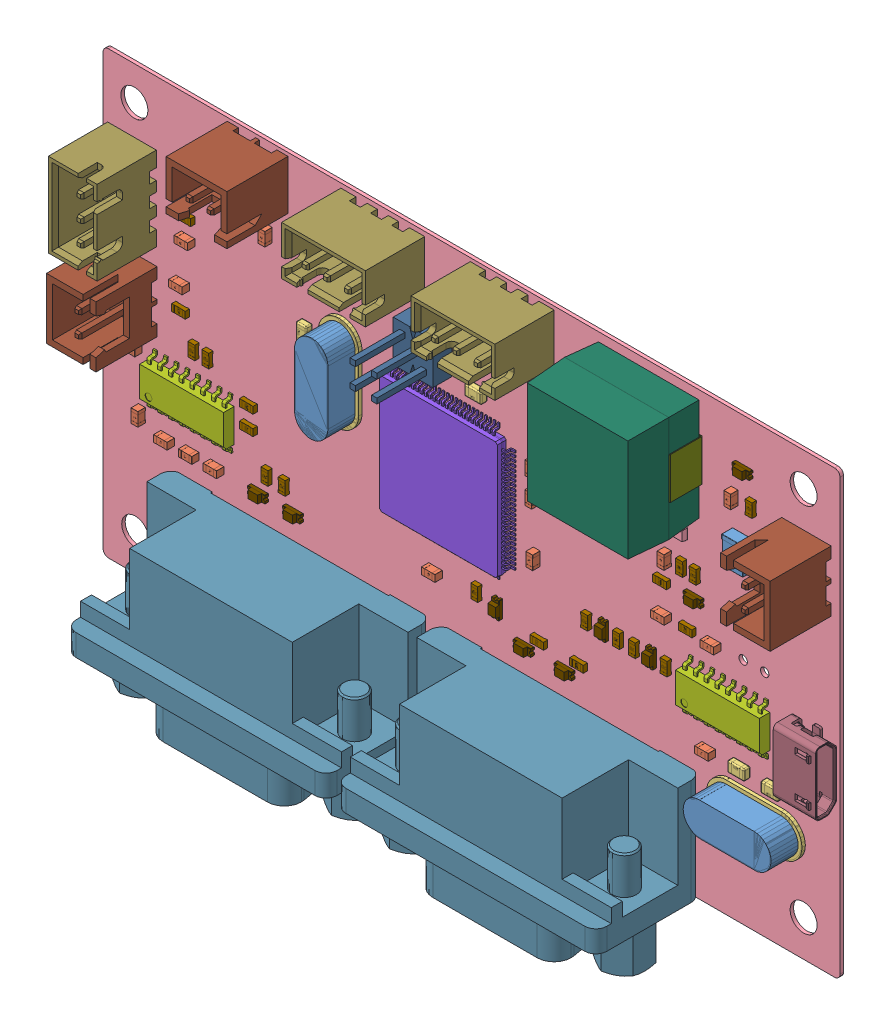
SolidWorks assembly Motor_Driver_Module, configuration Default. Lengths in mm.
Overall size (87 57.49 16.88).
208 component instances, 22 part files, 0 mates.
Components (placement in the parent):
- Motor_Driver_Module.step-1: Motor_Driver_Module.step [Default] at origin size (87 57.49 16.88)
  - X2.step-1: X2.step [Default] at origin size (11.27 4.77 5.6)
    - Xtal2.step-1: Xtal2.step [Default] at (353.2221 89.0021 0) x (-1 0 0) z (0 0 1) size (11.17 4.67 5.6)
      - User_Library-HC49S_Open_CASCADE_STEP_translator_6.2_316.2.step-1: User_Library-HC49S_Open_CASCADE_STEP_translator_6.2_316.2.step [Default] at origin size (11.17 4.67 5.6)
        - User_Library-HC49S_HC49S1.step-1: User_Library-HC49S_HC49S1.step [Default] at (0 0.0112 0.0127) size (11.17 4.67 5.6)
          - User_Library-HC49S_Open_CASCADE_STEP_translator_6.2_282.2.step-1: User_Library-HC49S_Open_CASCADE_STEP_translator_6.2_282.2.step [Default] at origin size (11.17 4.67 5.6)
            - User_Library-HC49S_340979409.step-1: User_Library-HC49S_340979409.step [Default] at (2.575 0.0126 0.0127) size (10.27 3.84 3.6)
              - User_Library-HC49S_Extruded3.step-1: User_Library-HC49S_Extruded3.step [Default] at origin size (10.27 3.84 3.6)
            - User_Library-HC49S_340739185.step-1: User_Library-HC49S_340739185.step [Default] at (-0.0117 -0.0104 -1.9873) size (0.43 0.43 2.1)
              - User_Library-HC49S_Cylinder1.step-1: User_Library-HC49S_Cylinder1.step [Default] at origin size (0.43 0.43 2.1)
            - User_Library-HC49S_340739185.step-2: User_Library-HC49S_340739185.step [Default] at (4.9883 -0.0104 -1.9873) size (0.43 0.43 2.1)
              - User_Library-HC49S_Cylinder1.step-1: User_Library-HC49S_Cylinder1.step [Default] at origin size (0.43 0.43 2.1)
            - User_Library-HC49S_340978513.step-1: User_Library-HC49S_340978513.step [Default] at (2.575 0 0.0127) size (11.17 4.67 0.4)
              - User_Library-HC49S_Extruded2.step-1: User_Library-HC49S_Extruded2.step [Default] at origin size (11.17 4.67 0.4)
    - Xtal2.step-2: Xtal2.step [Default] at (353.1221 89.1021 0) x (-1 0 0) z (0 0 1) size (11.17 4.67 5.6)
      - User_Library-HC49S_Open_CASCADE_STEP_translator_6.2_316.2.step-1: User_Library-HC49S_Open_CASCADE_STEP_translator_6.2_316.2.step [Default] at origin size (11.17 4.67 5.6)
        - User_Library-HC49S_HC49S1.step-1: User_Library-HC49S_HC49S1.step [Default] at (0 0.0112 0.0127) size (11.17 4.67 5.6)
          - User_Library-HC49S_Open_CASCADE_STEP_translator_6.2_282.2.step-1: User_Library-HC49S_Open_CASCADE_STEP_translator_6.2_282.2.step [Default] at origin size (11.17 4.67 5.6)
            - User_Library-HC49S_340979409.step-1: User_Library-HC49S_340979409.step [Default] at (2.575 0.0126 0.0127) size (10.27 3.84 3.6)
              - User_Library-HC49S_Extruded3.step-1: User_Library-HC49S_Extruded3.step [Default] at origin size (10.27 3.84 3.6)
            - User_Library-HC49S_340739185.step-1: User_Library-HC49S_340739185.step [Default] at (-0.0117 -0.0104 -1.9873) size (0.43 0.43 2.1)
              - User_Library-HC49S_Cylinder1.step-1: User_Library-HC49S_Cylinder1.step [Default] at origin size (0.43 0.43 2.1)
            - User_Library-HC49S_340739185.step-2: User_Library-HC49S_340739185.step [Default] at (4.9883 -0.0104 -1.9873) size (0.43 0.43 2.1)
              - User_Library-HC49S_Cylinder1.step-1: User_Library-HC49S_Cylinder1.step [Default] at origin size (0.43 0.43 2.1)
            - User_Library-HC49S_340978513.step-1: User_Library-HC49S_340978513.step [Default] at (2.575 0 0.0127) size (11.17 4.67 0.4)
              - User_Library-HC49S_Extruded2.step-1: User_Library-HC49S_Extruded2.step [Default] at origin size (11.17 4.67 0.4)
  - X1.step-1: X1.step [Default] at origin size (4.77 11.27 5.6)
    - Xtal2.step-1: Xtal2.step [Default] at (301.4731 107.5069 0) x (0 1 0) z (0 0 1) size (11.17 4.67 5.6)
      - User_Library-HC49S_Open_CASCADE_STEP_translator_6.2_316.2.step-1: User_Library-HC49S_Open_CASCADE_STEP_translator_6.2_316.2.step [Default] at origin size (11.17 4.67 5.6)
        - User_Library-HC49S_HC49S1.step-1: User_Library-HC49S_HC49S1.step [Default] at (0 0.0112 0.0127) size (11.17 4.67 5.6)
          - User_Library-HC49S_Open_CASCADE_STEP_translator_6.2_282.2.step-1: User_Library-HC49S_Open_CASCADE_STEP_translator_6.2_282.2.step [Default] at origin size (11.17 4.67 5.6)
            - User_Library-HC49S_340979409.step-1: User_Library-HC49S_340979409.step [Default] at (2.575 0.0126 0.0127) size (10.27 3.84 3.6)
              - User_Library-HC49S_Extruded3.step-1: User_Library-HC49S_Extruded3.step [Default] at origin size (10.27 3.84 3.6)
            - User_Library-HC49S_340739185.step-1: User_Library-HC49S_340739185.step [Default] at (-0.0117 -0.0104 -1.9873) size (0.43 0.43 2.1)
              - User_Library-HC49S_Cylinder1.step-1: User_Library-HC49S_Cylinder1.step [Default] at origin size (0.43 0.43 2.1)
            - User_Library-HC49S_340739185.step-2: User_Library-HC49S_340739185.step [Default] at (4.9883 -0.0104 -1.9873) size (0.43 0.43 2.1)
              - User_Library-HC49S_Cylinder1.step-1: User_Library-HC49S_Cylinder1.step [Default] at origin size (0.43 0.43 2.1)
            - User_Library-HC49S_340978513.step-1: User_Library-HC49S_340978513.step [Default] at (2.575 0 0.0127) size (11.17 4.67 0.4)
              - User_Library-HC49S_Extruded2.step-1: User_Library-HC49S_Extruded2.step [Default] at origin size (11.17 4.67 0.4)
    - Xtal2.step-2: Xtal2.step [Default] at (301.5731 107.6069 0) x (0 1 0) z (0 0 1) size (11.17 4.67 5.6)
      - User_Library-HC49S_Open_CASCADE_STEP_translator_6.2_316.2.step-1: User_Library-HC49S_Open_CASCADE_STEP_translator_6.2_316.2.step [Default] at origin size (11.17 4.67 5.6)
        - User_Library-HC49S_HC49S1.step-1: User_Library-HC49S_HC49S1.step [Default] at (0 0.0112 0.0127) size (11.17 4.67 5.6)
          - User_Library-HC49S_Open_CASCADE_STEP_translator_6.2_282.2.step-1: User_Library-HC49S_Open_CASCADE_STEP_translator_6.2_282.2.step [Default] at origin size (11.17 4.67 5.6)
            - User_Library-HC49S_340979409.step-1: User_Library-HC49S_340979409.step [Default] at (2.575 0.0126 0.0127) size (10.27 3.84 3.6)
              - User_Library-HC49S_Extruded3.step-1: User_Library-HC49S_Extruded3.step [Default] at origin size (10.27 3.84 3.6)
            - User_Library-HC49S_340739185.step-1: User_Library-HC49S_340739185.step [Default] at (-0.0117 -0.0104 -1.9873) size (0.43 0.43 2.1)
              - User_Library-HC49S_Cylinder1.step-1: User_Library-HC49S_Cylinder1.step [Default] at origin size (0.43 0.43 2.1)
            - User_Library-HC49S_340739185.step-2: User_Library-HC49S_340739185.step [Default] at (4.9883 -0.0104 -1.9873) size (0.43 0.43 2.1)
              - User_Library-HC49S_Cylinder1.step-1: User_Library-HC49S_Cylinder1.step [Default] at origin size (0.43 0.43 2.1)
            - User_Library-HC49S_340978513.step-1: User_Library-HC49S_340978513.step [Default] at (2.575 0 0.0127) size (11.17 4.67 0.4)
              - User_Library-HC49S_Extruded2.step-1: User_Library-HC49S_Extruded2.step [Default] at origin size (11.17 4.67 0.4)
  - U4.step-1: U4.step [Default] at origin size (1.6 1.6 0.6)
    - 5616371456.step-1: 5616371456.step [Default] at (341.503 113.886 0.005) x (0 -1 0) z (0 0 1) size (1.6 1.6 0.6)
      - Body.step-1: Body.step [Default] at origin size (1.2 1.6 0.6)
      - PinsArrayL.step-1: PinsArrayL.step [Default] at origin size (0.3 1.21 0.07)
      - PinsArrayR.step-1: PinsArrayR.step [Default] at origin size (0.3 1.21 0.07)
  - U3.step-1: U3.step [Default] at origin size (9.9 6 1.4)
    - SOIC-16.step-1: SOIC-16.step [Default] at (283.9719 98.3311 0) x (0 1 0) z (1 0 0) size (6 1.4 9.9)
  - U2.step-1: U2.step [Default] at origin size (9.9 6 1.4)
    - SOIC-16.step-1: SOIC-16.step [Default] at (347.2179 98.6791 0) x (0 1 0) z (1 0 0) size (6 1.4 9.9)
  - U1.step-1: U1.step [Default] at origin size (16 16 1.2)
    - ATMEGA2560-16AU--3DModel-STEP-56544.step-1: ATMEGA2560-16AU--3DModel-STEP-56544.step [Default] at (314.071 106.1719 0.65) x (0 -1 0) z (-1 0 0) size (16 1.2 16)
  - R23.step-1: R23.step [Default] at origin size (0.81 1.6 0.51)
    - User_Library-User_Library-res0603_res0603_body.step-1: User_Library-User_Library-res0603_res0603_body.step [Default] at (343.4 110.4 0) x (0 1 0) z (0 0 1) size (1.6 0.81 0.51)
  - R22.step-1: R22.step [Default] at origin size (0.81 1.6 0.51)
    - User_Library-User_Library-res0603_res0603_body.step-1: User_Library-User_Library-res0603_res0603_body.step [Default] at (341.8 110.4 0) x (0 -1 0) z (0 0 1) size (1.6 0.81 0.51)
  - R21.step-1: R21.step [Default] at origin size (1.6 0.81 0.51)
    - User_Library-User_Library-res0603_res0603_body.step-1: User_Library-User_Library-res0603_res0603_body.step [Default] at (339.5 107.8 0) x (-1 0 0) z (0 0 1) size (1.6 0.81 0.51)
  - R20.step-1: R20.step [Default] at origin size (1.6 0.81 0.51)
    - User_Library-User_Library-res0603_res0603_body.step-1: User_Library-User_Library-res0603_res0603_body.step [Default] at (290.703 99.06 0) x (1 0 0) z (0 0 1) size (1.6 0.81 0.51)
  - R19.step-1: R19.step [Default] at origin size (1.6 0.81 0.51)
    - User_Library-User_Library-res0603_res0603_body.step-1: User_Library-User_Library-res0603_res0603_body.step [Default] at (290.703 101.346 0) x (1 0 0) z (0 0 1) size (1.6 0.81 0.51)
  - R18.step-1: R18.step [Default] at origin size (0.81 1.6 0.51)
    - User_Library-User_Library-res0603_res0603_body.step-1: User_Library-User_Library-res0603_res0603_body.step [Default] at (284.226 103.771 0) x (0 1 0) z (0 0 1) size (1.6 0.81 0.51)
  - R17.step-1: R17.step [Default] at origin size (0.81 1.6 0.51)
    - User_Library-User_Library-res0603_res0603_body.step-1: User_Library-User_Library-res0603_res0603_body.step [Default] at (285.877 103.759 0) x (0 1 0) z (0 0 1) size (1.6 0.81 0.51)
  - R16.step-1: R16.step [Default] at origin size (0.81 1.6 0.51)
    - User_Library-User_Library-res0603_res0603_body.step-1: User_Library-User_Library-res0603_res0603_body.step [Default] at (330.6 99.314 0) x (0 1 0) z (0 0 1) size (1.6 0.81 0.51)
  - R15.step-1: R15.step [Default] at origin size (0.81 1.6 0.51)
    - User_Library-User_Library-res0603_res0603_body.step-1: User_Library-User_Library-res0603_res0603_body.step [Default] at (336.2274 99.314 0) x (0 1 0) z (0 0 1) size (1.6 0.81 0.51)
  - R14.step-1: R14.step [Default] at origin size (0.81 1.6 0.51)
    - User_Library-User_Library-res0603_res0603_body.step-1: User_Library-User_Library-res0603_res0603_body.step [Default] at (339.979 99.314 0) x (0 1 0) z (0 0 1) size (1.6 0.81 0.51)
  - R13.step-1: R13.step [Default] at origin size (0.81 1.6 0.51)
    - User_Library-User_Library-res0603_res0603_body.step-1: User_Library-User_Library-res0603_res0603_body.step [Default] at (334.3516 99.314 0) x (0 1 0) z (0 0 1) size (1.6 0.81 0.51)
  - R12.step-1: R12.step [Default] at origin size (0.81 1.6 0.51)
    - User_Library-User_Library-res0603_res0603_body.step-1: User_Library-User_Library-res0603_res0603_body.step [Default] at (317.627 95.758 0) x (0 1 0) z (0 0 1) size (1.6 0.81 0.51)
  - R11.step-1: R11.step [Default] at origin size (1.6 0.81 0.51)
    - User_Library-User_Library-res0603_res0603_body.step-1: User_Library-User_Library-res0603_res0603_body.step [Default] at (342.519 104.394 0) x (-1 0 0) z (0 0 1) size (1.6 0.81 0.51)
  - R10.step-1: R10.step [Default] at origin size (0.81 1.6 0.51)
    - User_Library-User_Library-res0603_res0603_body.step-1: User_Library-User_Library-res0603_res0603_body.step [Default] at (290.322 119.773 0) x (0 -1 0) z (0 0 1) size (1.6 0.81 0.51)
  - R9.step-1: R9.step [Default] at origin size (1.6 0.81 0.51)
    - User_Library-User_Library-res0603_res0603_body.step-1: User_Library-User_Library-res0603_res0603_body.step [Default] at (282.702 107.061 0) x (1 0 0) z (0 0 1) size (1.6 0.81 0.51)
  - R8.step-1: R8.step [Default] at origin size (0.81 1.6 0.51)
    - User_Library-User_Library-res0603_res0603_body.step-1: User_Library-User_Library-res0603_res0603_body.step [Default] at (321.691 120.777 0) x (0 -1 0) z (0 0 1) size (1.6 0.81 0.51)
  - R7.step-1: R7.step [Default] at origin size (1.6 0.81 0.51)
    - User_Library-User_Library-res0603_res0603_body.step-1: User_Library-User_Library-res0603_res0603_body.step [Default] at (283.337 116.84 0) x (1 0 0) z (0 0 1) size (1.6 0.81 0.51)
  - R6.step-1: R6.step [Default] at origin size (0.81 1.6 0.51)
    - User_Library-User_Library-res0603_res0603_body.step-1: User_Library-User_Library-res0603_res0603_body.step [Default] at (306.197 119.988 0) x (0 -1 0) z (0 0 1) size (1.6 0.81 0.51)
  - R5.step-1: R5.step [Default] at origin size (0.81 1.6 0.51)
    - User_Library-User_Library-res0603_res0603_body.step-1: User_Library-User_Library-res0603_res0603_body.step [Default] at (350.012 120.535 0) x (0 -1 0) z (0 0 1) size (1.6 0.81 0.51)
  - R4.step-1: R4.step [Default] at origin size (1.6 0.81 0.51)
    - User_Library-User_Library-res0603_res0603_body.step-1: User_Library-User_Library-res0603_res0603_body.step [Default] at (324.993 94.361 0) x (1 0 0) z (0 0 1) size (1.6 0.81 0.51)
  - R3.step-1: R3.step [Default] at origin size (1.6 0.81 0.51)
    - User_Library-User_Library-res0603_res0603_body.step-1: User_Library-User_Library-res0603_res0603_body.step [Default] at (329.692 94.361 0) x (1 0 0) z (0 0 1) size (1.6 0.81 0.51)
  - R2.step-1: R2.step [Default] at origin size (0.81 1.6 0.51)
    - User_Library-User_Library-res0603_res0603_body.step-1: User_Library-User_Library-res0603_res0603_body.step [Default] at (292.862 95.25 0) x (0 1 0) z (0 0 1) size (1.6 0.81 0.51)
  - R1.step-1: R1.step [Default] at origin size (0.81 1.6 0.51)
    - User_Library-User_Library-res0603_res0603_body.step-1: User_Library-User_Library-res0603_res0603_body.step [Default] at (294.894 95.25 0) x (0 1 0) z (0 0 1) size (1.6 0.81 0.51)
  - P10.step-1: P10.step [Default] at origin size (4.67 4.88 11.18)
    - 70042464.step-1: 70042464.step [Default] at (312.2929 118.618 2.4) x (-1 0 0) z (0 0 1) size (4.67 4.88 11.18)
  - P9.step-1: P9.step [Default] at origin size (7.17 5.84 10.21)
    - JST_-_XH_-_Thru_-_2Pin_-_2.5mm_(Genuine).step-1: JST_-_XH_-_Thru_-_2Pin_-_2.5mm_(Genuine).step [Default] at (291.5465 125.5267 0) x (1 0 0) z (0 0 1) size (7.17 5.84 10.21)
  - P8.step-1: P8.step [Default] at origin size (5.84 7.17 10.21)
    - JST_-_XH_-_Thru_-_2Pin_-_2.5mm_(Genuine).step-1: JST_-_XH_-_Thru_-_2Pin_-_2.5mm_(Genuine).step [Default] at (277.1903 106.2936 0) x (0 1 0) z (0 0 1) size (7.17 5.84 10.21)
  - P7.step-1: P7.step [Default] at origin size (5.84 7.17 10.21)
    - JST_-_XH_-_Thru_-_2Pin_-_2.5mm_(Genuine).step-1: JST_-_XH_-_Thru_-_2Pin_-_2.5mm_(Genuine).step [Default] at (355.9047 117.5204 0) x (0 -1 0) z (0 0 1) size (7.17 5.84 10.21)
  - P6.step-1: P6.step [Default] at origin size (9.9 5.75 10.4)
    - B3B-XH-A-LF--SN---3DModel-STEP-269445.step-1: B3B-XH-A-LF--SN---3DModel-STEP-269445.step [Default] at (324.1039 125.4796 0) x (-1 0 0) z (0 1 0) size (9.9 10.4 5.75)
  - P5.step-1: P5.step [Default] at origin size (5.75 9.9 10.4)
    - B3B-XH-A-LF--SN---3DModel-STEP-269445.step-1: B3B-XH-A-LF--SN---3DModel-STEP-269445.step [Default] at (277.2411 119.2999 0) x (0 -1 0) z (-1 0 0) size (9.9 10.4 5.75)
  - P4.step-1: P4.step [Default] at origin size (9.9 5.75 10.4)
    - B3B-XH-A-LF--SN---3DModel-STEP-269445.step-1: B3B-XH-A-LF--SN---3DModel-STEP-269445.step [Default] at (308.824 125.3526 0) x (-1 0 0) z (0 1 0) size (9.9 10.4 5.75)
  - P3.step-1: P3.step [Default] at origin size (5 7.8 2.7)
    - 2174507-2.step-1: 2174507-2.step [Default] at (359.9581 98.203 1.3) x (0 1 0) z (1 0 0) size (7.8 2.7 5)
  - P2.step-1: P2.step [Default] at origin size (30.81 18.3 16.88)
    - connector_a-df_09_a_kg-t2.step-1: connector_a-df_09_a_kg-t2.step [Default] at (296.688 77.6 6.2) x (1 0 0) z (0 -1 0) size (30.81 16.88 18.3)
  - P1.step-1: P1.step [Default] at origin size (30.81 18.3 16.88)
    - connector_a-df_09_a_kg-t2.step-1: connector_a-df_09_a_kg-t2.step [Default] at (328.5409 77.6 6.2) x (1 0 0) z (0 -1 0) size (30.81 16.88 18.3)
  - L1.step-1: L1.step [Default] at origin size (12.5 12.5 8.5)
    - 5616371840.step-1: 5616371840.step [Default] at (337.8199 122.3009 0) x (-1 0 0) z (0 0 1) size (12.5 12.5 8.5)
      - Chamfer.step-1: Chamfer.step [Default] at origin size (12.3 12.5 8.4)
      - FilletPin1.step-1: FilletPin1.step [Default] at origin size (2.05 4.9 3.88)
      - FilletPin2.step-1: FilletPin2.step [Default] at origin size (2.15 4.9 3.88)
  - D9.step-1: D9.step [Default] at origin size (2.06 0.91 0.84)
    - LED_0805.step-1: LED_0805.step [Default] at (344.0001 107.7999 0) x (0 -1 0) z (0 0 1) size (0.91 2.06 0.84)
  - D8.step-1: D8.step [Default] at origin size (0.91 2.06 0.84)
    - LED_0805.step-1: LED_0805.step [Default] at (332.5759 100.0981 0) x (1 0 0) z (0 0 1) size (0.91 2.06 0.84)
  - D7.step-1: D7.step [Default] at origin size (0.91 2.06 0.84)
    - LED_0805.step-1: LED_0805.step [Default] at (338.2032 100.0981 0) x (1 0 0) z (0 0 1) size (0.91 2.06 0.84)
  - D6.step-1: D6.step [Default] at origin size (0.91 2.06 0.84)
    - LED_0805.step-1: LED_0805.step [Default] at (320.0401 96.0501 0) x (1 0 0) z (0 0 1) size (0.91 2.06 0.84)
  - D5.step-1: D5.step [Default] at origin size (2.06 0.91 0.84)
    - LED_0805.step-1: LED_0805.step [Default] at (348.2249 123.8251 0) x (0 1 0) z (0 0 1) size (0.91 2.06 0.84)
  - D4.step-1: D4.step [Default] at origin size (2.06 0.91 0.84)
    - LED_0805.step-1: LED_0805.step [Default] at (322.4149 92.8371 0) x (0 1 0) z (0 0 1) size (0.91 2.06 0.84)
  - D3.step-1: D3.step [Default] at origin size (2.06 0.91 0.84)
    - LED_0805.step-1: LED_0805.step [Default] at (327.2409 92.8371 0) x (0 1 0) z (0 0 1) size (0.91 2.06 0.84)
  - D2.step-1: D2.step [Default] at origin size (2.06 0.91 0.84)
    - LED_0805.step-1: LED_0805.step [Default] at (291.0459 92.8371 0) x (0 1 0) z (0 0 1) size (0.91 2.06 0.84)
  - D1.step-1: D1.step [Default] at origin size (2.06 0.91 0.84)
    - LED_0805.step-1: LED_0805.step [Default] at (296.7101 92.8369 0) x (0 -1 0) z (0 0 1) size (0.91 2.06 0.84)
  - C28.step-1: C28.step [Default] at origin size (3.2 2.5 1.3)
    - User_Library-cap_1210_lowprofile.step-1: User_Library-cap_1210_lowprofile.step [Default] at (335.0259 113.7919 0) x (-1 0 0) z (0 0 1) size (3.2 2.5 1.3)
  - C27.step-1: C27.step [Default] at origin size (3.2 2.5 1.3)
    - User_Library-cap_1210_lowprofile.step-1: User_Library-cap_1210_lowprofile.step [Default] at (335.0259 110.3629 0) x (-1 0 0) z (0 0 1) size (3.2 2.5 1.3)
  - C26.step-1: C26.step [Default] at origin size (0.81 1.6 0.88)
    - User_Library-User_Library-cap0603_cap0603_body.step-1: User_Library-User_Library-cap0603_cap0603_body.step [Default] at (339.979 110.39 0) x (0 -1 0) z (0 0 1) size (1.6 0.81 0.88)
  - C25.step-1: C25.step [Default] at origin size (0.81 1.6 0.88)
    - User_Library-User_Library-cap0603_cap0603_body.step-1: User_Library-User_Library-cap0603_cap0603_body.step [Default] at (347.853 120.523 0) x (0 -1 0) z (0 0 1) size (1.6 0.81 0.88)
  - C24.step-1: C24.step [Default] at origin size (2.5 3.2 1.3)
    - User_Library-cap_1210_lowprofile.step-1: User_Library-cap_1210_lowprofile.step [Default] at (348.8689 115.5701 0) x (0 1 0) z (0 0 1) size (3.2 2.5 1.3)
  - C23.step-1: C23.step [Default] at origin size (0.81 1.6 0.88)
    - User_Library-User_Library-cap0603_cap0603_body.step-1: User_Library-User_Library-cap0603_cap0603_body.step [Default] at (339.0999 113.8 0) x (0 1 0) z (0 0 1) size (1.6 0.81 0.88)
  - C22.step-1: C22.step [Default] at origin size (1.6 0.81 0.88)
    - User_Library-User_Library-cap0603_cap0603_body.step-1: User_Library-User_Library-cap0603_cap0603_body.step [Default] at (283.845 92.964 0) x (-1 0 0) z (0 0 1) size (1.6 0.81 0.88)
  - C21.step-1: C21.step [Default] at origin size (1.6 0.81 0.88)
    - User_Library-User_Library-cap0603_cap0603_body.step-1: User_Library-User_Library-cap0603_cap0603_body.step [Default] at (286.766 92.964 0) x (-1 0 0) z (0 0 1) size (1.6 0.81 0.88)
  - C20.step-1: C20.step [Default] at origin size (0.81 1.6 0.88)
    - User_Library-User_Library-cap0603_cap0603_body.step-1: User_Library-User_Library-cap0603_cap0603_body.step [Default] at (277.8759 93.98 0) x (0 1 0) z (0 0 1) size (1.6 0.81 0.88)
  - C19.step-1: C19.step [Default] at origin size (1.6 0.81 0.88)
    - User_Library-User_Library-cap0603_cap0603_body.step-1: User_Library-User_Library-cap0603_cap0603_body.step [Default] at (277.114 100.584 0) x (1 0 0) z (0 0 1) size (1.6 0.81 0.88)
  - C18.step-1: C18.step [Default] at origin size (1.6 0.81 0.88)
    - User_Library-User_Library-cap0603_cap0603_body.step-1: User_Library-User_Library-cap0603_cap0603_body.step [Default] at (280.924 92.964 0) x (-1 0 0) z (0 0 1) size (1.6 0.81 0.88)
  - C17.step-1: C17.step [Default] at origin size (2 1.25 0.78)
    - 0805-SMD-Capacitor.step-1: 0805-SMD-Capacitor.step [Default] at (352.679 93.091 0) x (-1 0 0) z (0 1 0) size (2 0.78 1.25)
  - C16.step-1: C16.step [Default] at origin size (1.6 0.81 0.88)
    - User_Library-User_Library-cap0603_cap0603_body.step-1: User_Library-User_Library-cap0603_cap0603_body.step [Default] at (344.8051 93.091 0) x (1 0 0) z (0 0 1) size (1.6 0.81 0.88)
  - C15.step-1: C15.step [Default] at origin size (2 1.25 0.78)
    - 0805-SMD-Capacitor.step-1: 0805-SMD-Capacitor.step [Default] at (348.742 93.218 0) x (1 0 0) z (0 -1 0) size (2 0.78 1.25)
  - C14.step-1: C14.step [Default] at origin size (1.6 0.81 0.88)
    - User_Library-User_Library-cap0603_cap0603_body.step-1: User_Library-User_Library-cap0603_cap0603_body.step [Default] at (339.5981 104.394 0) x (1 0 0) z (0 0 1) size (1.6 0.81 0.88)
  - C13.step-1: C13.step [Default] at origin size (0.81 1.6 0.88)
    - User_Library-User_Library-cap0603_cap0603_body.step-1: User_Library-User_Library-cap0603_cap0603_body.step [Default] at (324.358 111.887 0) x (0 1 0) z (0 0 1) size (1.6 0.81 0.88)
  - C12.step-1: C12.step [Default] at origin size (0.81 1.6 0.88)
    - User_Library-User_Library-cap0603_cap0603_body.step-1: User_Library-User_Library-cap0603_cap0603_body.step [Default] at (324.358 108.839 0) x (0 1 0) z (0 0 1) size (1.6 0.81 0.88)
  - C11.step-1: C11.step [Default] at origin size (0.81 1.6 0.88)
    - User_Library-User_Library-cap0603_cap0603_body.step-1: User_Library-User_Library-cap0603_cap0603_body.step [Default] at (324.485 102.616 0) x (0 -1 0) z (0 0 1) size (1.6 0.81 0.88)
  - C10.step-1: C10.step [Default] at origin size (1.6 0.81 0.88)
    - User_Library-User_Library-cap0603_cap0603_body.step-1: User_Library-User_Library-cap0603_cap0603_body.step [Default] at (312.547 95.25 0) x (-1 0 0) z (0 0 1) size (1.6 0.81 0.88)
  - C9.step-1: C9.step [Default] at origin size (2 1.25 0.78)
    - 0805-SMD-Capacitor.step-1: 0805-SMD-Capacitor.step [Default] at (317.7 116.2 0) x (-1 0 0) z (0 1 0) size (2 0.78 1.25)
  - C8.step-1: C8.step [Default] at origin size (1.6 0.81 0.88)
    - User_Library-User_Library-cap0603_cap0603_body.step-1: User_Library-User_Library-cap0603_cap0603_body.step [Default] at (345.44 104.267 0) x (-1 0 0) z (0 0 1) size (1.6 0.81 0.88)
  - C7.step-1: C7.step [Default] at origin size (1.25 2 0.78)
    - 0805-SMD-Capacitor.step-1: 0805-SMD-Capacitor.step [Default] at (297.434 107.415 0) x (0 -1 0) z (-1 0 0) size (2 0.78 1.25)
  - C6.step-1: C6.step [Default] at origin size (1.25 2 0.78)
    - 0805-SMD-Capacitor.step-1: 0805-SMD-Capacitor.step [Default] at (297.434 112.241 0) x (0 1 0) z (1 0 0) size (2 0.78 1.25)
  - C5.step-1: C5.step [Default] at origin size (0.81 1.6 0.88)
    - User_Library-User_Library-cap0603_cap0603_body.step-1: User_Library-User_Library-cap0603_cap0603_body.step [Default] at (292.862 119.888 0) x (0 1 0) z (0 0 1) size (1.6 0.81 0.88)
  - C4.step-1: C4.step [Default] at origin size (1.6 0.81 0.88)
    - User_Library-User_Library-cap0603_cap0603_body.step-1: User_Library-User_Library-cap0603_cap0603_body.step [Default] at (282.7021 109.728 0) x (1 0 0) z (0 0 1) size (1.6 0.81 0.88)
  - C3.step-1: C3.step [Default] at origin size (1.6 0.81 0.88)
    - User_Library-User_Library-cap0603_cap0603_body.step-1: User_Library-User_Library-cap0603_cap0603_body.step [Default] at (283.337 114.554 0) x (1 0 0) z (0 0 1) size (1.6 0.81 0.88)
  - C2.step-1: C2.step [Default] at origin size (0.81 1.6 0.88)
    - User_Library-User_Library-cap0603_cap0603_body.step-1: User_Library-User_Library-cap0603_cap0603_body.step [Default] at (319.024 120.904 0) x (0 -1 0) z (0 0 1) size (1.6 0.81 0.88)
  - C1.step-1: C1.step [Default] at origin size (0.81 1.6 0.88)
    - User_Library-User_Library-cap0603_cap0603_body.step-1: User_Library-User_Library-cap0603_cap0603_body.step [Default] at (303.911 120.015 0) x (0 -1 0) z (0 0 1) size (1.6 0.81 0.88)
  - Board.step-1: Board.step [Default] at origin size (87 52.07 0.41)
